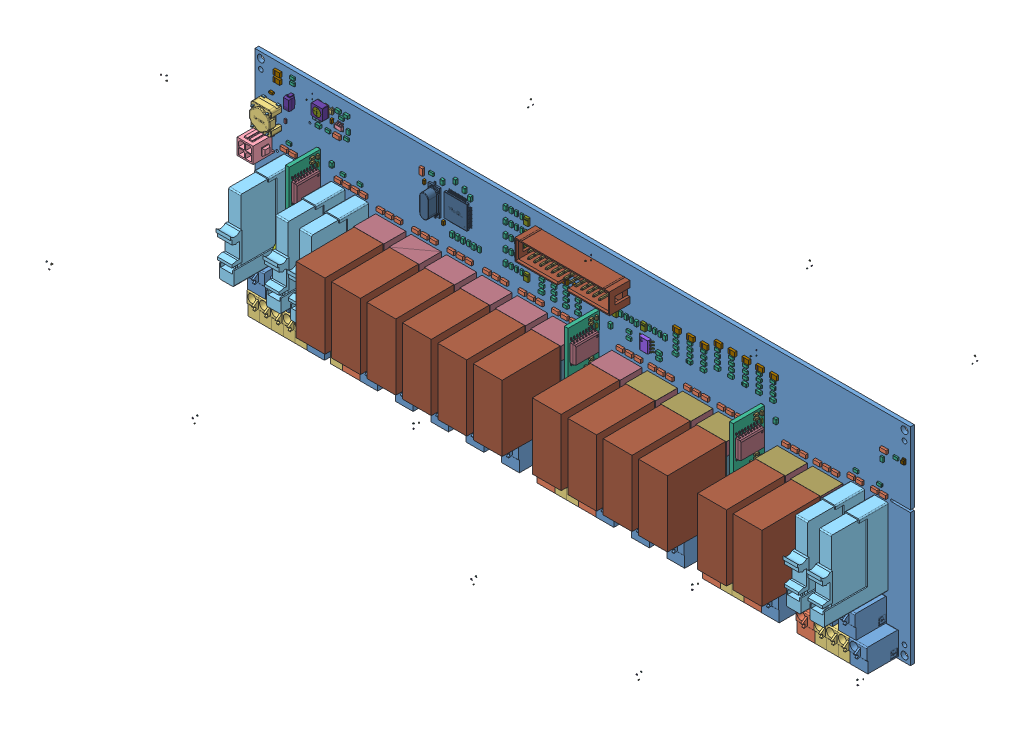
SolidWorks assembly _SC940D, configuration Default. Lengths in mm. (continued)
Components (placement in the parent): (continued)
- T25-1: T25 [Default] at origin size (306.6 73.44 23.48)
  - SW3dPS-transistor_SOT233_4-1: SW3dPS-transistor_SOT233_4 [Default] at (303.1237 70.5668 -21.9) x (1 0 0) z (0 -1 0) size (2.9 1.1 1.6)
  - SW3dPS-transistor_SOT233_5-1: SW3dPS-transistor_SOT233_5 [Default] at (0.3031 0.0706 -0.0219) x (1 0 0) z (0 -1 0) size (2.18 2.18 2.18)
  - SW3dPS-transistor_SOT233_6-1: SW3dPS-transistor_SOT233_6 [Default] at (0.0003 0.0001 0) x (1 0 0) z (0 -1 0) size (2.18 2.18 2.18)
  - SW3dPS-transistor_SOT233_7-1: SW3dPS-transistor_SOT233_7 [Default] x (1 0 0) z (0 -1 0) size (2.18 2.18 2.18)
- T24-1: T24 [Default] at origin size (298.98 73.44 23.48)
  - SW3dPS-transistor_SOT233_4-1: SW3dPS-transistor_SOT233_4 [Default] at (295.5037 70.5668 -21.9) x (1 0 0) z (0 -1 0) size (2.9 1.1 1.6)
  - SW3dPS-transistor_SOT233_5-1: SW3dPS-transistor_SOT233_5 [Default] at (0.2955 0.0706 -0.0219) x (1 0 0) z (0 -1 0) size (2.18 2.18 2.18)
  - SW3dPS-transistor_SOT233_6-1: SW3dPS-transistor_SOT233_6 [Default] at (0.0003 0.0001 0) x (1 0 0) z (0 -1 0) size (2.18 2.18 2.18)
  - SW3dPS-transistor_SOT233_7-1: SW3dPS-transistor_SOT233_7 [Default] x (1 0 0) z (0 -1 0) size (2.18 2.18 2.18)
- T27-1: T27 [Default] at origin size (320.25 73.44 23.48)
  - SW3dPS-transistor_SOT233_4-1: SW3dPS-transistor_SOT233_4 [Default] at (316.7762 70.5668 -21.9) x (1 0 0) z (0 -1 0) size (2.9 1.1 1.6)
  - SW3dPS-transistor_SOT233_5-1: SW3dPS-transistor_SOT233_5 [Default] at (0.3168 0.0706 -0.0219) x (1 0 0) z (0 -1 0) size (2.18 2.18 2.18)
  - SW3dPS-transistor_SOT233_6-1: SW3dPS-transistor_SOT233_6 [Default] at (0.0003 0.0001 0) x (1 0 0) z (0 -1 0) size (2.18 2.18 2.18)
  - SW3dPS-transistor_SOT233_7-1: SW3dPS-transistor_SOT233_7 [Default] x (1 0 0) z (0 -1 0) size (2.18 2.18 2.18)
- T26-1: T26 [Default] at origin size (312.63 73.44 23.48)
  - SW3dPS-transistor_SOT233_4-1: SW3dPS-transistor_SOT233_4 [Default] at (309.1562 70.5668 -21.9) x (1 0 0) z (0 -1 0) size (2.9 1.1 1.6)
  - SW3dPS-transistor_SOT233_5-1: SW3dPS-transistor_SOT233_5 [Default] at (0.3092 0.0706 -0.0219) x (1 0 0) z (0 -1 0) size (2.18 2.18 2.18)
  - SW3dPS-transistor_SOT233_6-1: SW3dPS-transistor_SOT233_6 [Default] at (0.0003 0.0001 0) x (1 0 0) z (0 -1 0) size (2.18 2.18 2.18)
  - SW3dPS-transistor_SOT233_7-1: SW3dPS-transistor_SOT233_7 [Default] x (1 0 0) z (0 -1 0) size (2.18 2.18 2.18)
- D42-1: D42 [Default] at origin size (185.97 29.62 23.48)
  - SW3dPS-transistor_SOT233_4-1: SW3dPS-transistor_SOT233_4 [Default] at (182.6513 26.7469 -21.9) x (-1 0 0) z (0 1 0) size (2.9 1.1 1.6)
  - SW3dPS-transistor_SOT233_5-1: SW3dPS-transistor_SOT233_5 [Default] at (0.1827 0.0267 -0.0219) x (-1 0 0) z (0 1 0) size (2.18 2.18 2.18)
  - SW3dPS-transistor_SOT233_6-1: SW3dPS-transistor_SOT233_6 [Default] at (0.0002 0 0) x (-1 0 0) z (0 1 0) size (2.18 2.18 2.18)
  - SW3dPS-transistor_SOT233_7-1: SW3dPS-transistor_SOT233_7 [Default] x (-1 0 0) z (0 1 0) size (2.18 2.18 2.18)
- D43-1: D43 [Default] at origin size (196.12 29.62 23.48)
  - SW3dPS-transistor_SOT233_4-1: SW3dPS-transistor_SOT233_4 [Default] at (192.8113 26.7469 -21.9) x (-1 0 0) z (0 1 0) size (2.9 1.1 1.6)
  - SW3dPS-transistor_SOT233_5-1: SW3dPS-transistor_SOT233_5 [Default] at (0.1928 0.0267 -0.0219) x (-1 0 0) z (0 1 0) size (2.18 2.18 2.18)
  - SW3dPS-transistor_SOT233_6-1: SW3dPS-transistor_SOT233_6 [Default] at (0.0002 0 0) x (-1 0 0) z (0 1 0) size (2.18 2.18 2.18)
  - SW3dPS-transistor_SOT233_7-1: SW3dPS-transistor_SOT233_7 [Default] x (-1 0 0) z (0 1 0) size (2.18 2.18 2.18)
- R74-1: R74 [Default] at origin size (2 1.2 0.7)
  - RESC2012X70N-1: RESC2012X70N [Default] at (253.2061 52.7049 0) x (-1 0 0) z (0 1 0) size (2 0.7 1.2)
- R75-1: R75 [Default] at origin size (2 1.2 0.7)
  - RESC2012X70N-1: RESC2012X70N [Default] at (263.3662 52.7049 0) x (-1 0 0) z (0 1 0) size (2 0.7 1.2)
- T28-1: T28 [Default] at origin size (327.08 75.5 23.48)
  - SW3dPS-transistor_SOT233_4-1: SW3dPS-transistor_SOT233_4 [Default] at (323.6024 72.6306 -21.9) x (1 0 0) z (0 -1 0) size (2.9 1.1 1.6)
  - SW3dPS-transistor_SOT233_5-1: SW3dPS-transistor_SOT233_5 [Default] at (0.3236 0.0726 -0.0219) x (1 0 0) z (0 -1 0) size (2.18 2.18 2.18)
  - SW3dPS-transistor_SOT233_6-1: SW3dPS-transistor_SOT233_6 [Default] at (0.0003 0.0001 0) x (1 0 0) z (0 -1 0) size (2.18 2.18 2.18)
  - SW3dPS-transistor_SOT233_7-1: SW3dPS-transistor_SOT233_7 [Default] x (1 0 0) z (0 -1 0) size (2.18 2.18 2.18)
- T29-1: T29 [Default] at origin size (337.24 75.5 23.48)
  - SW3dPS-transistor_SOT233_4-1: SW3dPS-transistor_SOT233_4 [Default] at (333.7624 72.6306 -21.9) x (1 0 0) z (0 -1 0) size (2.9 1.1 1.6)
  - SW3dPS-transistor_SOT233_5-1: SW3dPS-transistor_SOT233_5 [Default] at (0.3338 0.0726 -0.0219) x (1 0 0) z (0 -1 0) size (2.18 2.18 2.18)
  - SW3dPS-transistor_SOT233_6-1: SW3dPS-transistor_SOT233_6 [Default] at (0.0003 0.0001 0) x (1 0 0) z (0 -1 0) size (2.18 2.18 2.18)
  - SW3dPS-transistor_SOT233_7-1: SW3dPS-transistor_SOT233_7 [Default] x (1 0 0) z (0 -1 0) size (2.18 2.18 2.18)
- D7_1-1: D7_1 [Default] at origin size (64.67 29.62 23.48)
  - SW3dPS-transistor_SOT233_4-1: SW3dPS-transistor_SOT233_4 [Default] at (-61.1887 26.7469 -21.9) x (-1 0 0) z (0 1 0) size (2.9 1.1 1.6)
  - SW3dPS-transistor_SOT233_5-1: SW3dPS-transistor_SOT233_5 [Default] at (-0.0612 0.0267 -0.0219) x (-1 0 0) z (0 1 0) size (2.18 2.18 2.18)
  - SW3dPS-transistor_SOT233_6-1: SW3dPS-transistor_SOT233_6 [Default] at (-0.0001 0 0) x (-1 0 0) z (0 1 0) size (2.18 2.18 2.18)
  - SW3dPS-transistor_SOT233_7-1: SW3dPS-transistor_SOT233_7 [Default] x (-1 0 0) z (0 1 0) size (2.18 2.18 2.18)
- R6-1: R6 [Default] at origin size (2 1.2 0.7)
  - RESC2012X70N-1: RESC2012X70N [Default] at (9.3662 52.7049 0) x (-1 0 0) z (0 1 0) size (2 0.7 1.2)
- T1-1: T1 [Default] at origin size (83.24 75.5 23.48)
  - SW3dPS-transistor_SOT233_4-1: SW3dPS-transistor_SOT233_4 [Default] at (79.7624 72.6306 -21.9) x (1 0 0) z (0 -1 0) size (2.9 1.1 1.6)
  - SW3dPS-transistor_SOT233_5-1: SW3dPS-transistor_SOT233_5 [Default] at (0.0798 0.0726 -0.0219) x (1 0 0) z (0 -1 0) size (2.18 2.18 2.18)
  - SW3dPS-transistor_SOT233_6-1: SW3dPS-transistor_SOT233_6 [Default] at (0.0001 0.0001 0) x (1 0 0) z (0 -1 0) size (2.18 2.18 2.18)
  - SW3dPS-transistor_SOT233_7-1: SW3dPS-transistor_SOT233_7 [Default] x (1 0 0) z (0 -1 0) size (2.18 2.18 2.18)
- U7-1: U7 [Default] at origin size (27.38 148.76 148.76)
  - SC943-0C_20-12-2012-1: SC943-0C_20-12-2012 [Default] at (213.4696 28.0022 3.7281) x (0 1 0.000663) z (1 0 0) size (148.66 148.66 27.38)
    - Board_1-1: Board_1 [Default] at (0 0 -1.6167) size (43.5 16.8 1.62)
    - R15-1: R15 [Default] at origin size (1.6 0.8 0.55)
      - RESC1608X84N_1-1: RESC1608X84N_1 [Default] at (-0.0001 1.9049 0) x (-1 0 0) z (0 1 0) size (1.6 0.55 0.8)
    - R11-1: R11 [Default] at origin size (2 1.2 0.7)
      - RESC2012X70N_1-1: RESC2012X70N_1 [Default] at (-3.6513 -0.4763 0) x (-1 0 0) z (0 1 0) size (2 0.7 1.2)
    - R7-1: R7 [Default] at origin size (2 1.2 0.7)
      - RESC2012X70N_1-1: RESC2012X70N_1 [Default] at (-5.2388 1.5874 0) x (-1 0 0) z (0 1 0) size (2 0.7 1.2)
    - D3-1: D3 [Default] at origin size (2.6 5.2 2.43)
      - SW3dPS-DO-214AC_SMA-1: SW3dPS-DO-214AC_SMA [Default] at (-1.4287 0.3175 -2.9167) x (1 0 0) z (0 0 -1) size (2.6 5.2 2.43)
    - T4-1: T4 [Default] at origin size (6.54 9.94 2.42)
      - SW3dPS-DPAK-1-1: SW3dPS-DPAK-1 [Default] at (10.9238 2.2758 -2.8167) x (1 0 0) z (0 1 0) size (6.54 2.42 9.94)
    - T3-1: T3 [Default] at origin size (6.54 9.94 2.42)
      - SW3dPS-DPAK-1-1: SW3dPS-DPAK-1 [Default] at (-10.3487 2.2758 -2.8167) x (1 0 0) z (0 1 0) size (6.54 2.42 9.94)
    - D5-1: D5 [Default] at origin size (2.6 5.2 2.43)
      - SW3dPS-DO-214AC_SMA-1: SW3dPS-DO-214AC_SMA [Default] at (2.0638 0.3175 -2.9167) x (1 0 0) z (0 0 -1) size (2.6 5.2 2.43)
    - D4-1: D4 [Default] at origin size (2.6 5.2 2.43)
      - SW3dPS-DO-214AC_SMA-1: SW3dPS-DO-214AC_SMA [Default] at (5.2388 0.3175 -2.9167) x (1 0 0) z (0 0 -1) size (2.6 5.2 2.43)
    - D2-1: D2 [Default] at origin size (2.6 5.2 2.43)
      - SW3dPS-DO-214AC_SMA-1: SW3dPS-DO-214AC_SMA [Default] at (-4.6037 0.3175 -2.9167) x (1 0 0) z (0 0 -1) size (2.6 5.2 2.43)
    - R25-1: R25 [Default] at origin size (3.2 1.6 0.84)
      - RESC3216X84N-1: RESC3216X84N [Default] at (-2.0851 5.5563 -1.6167) x (-1 0 0) z (0 -1 0) size (3.2 0.84 1.6)
    - R26-1: R26 [Default] at origin size (3.2 1.6 0.84)
      - RESC3216X84N-1: RESC3216X84N [Default] at (2.6989 5.5562 -1.6167) x (1 0 0) z (0 1 0) size (3.2 0.84 1.6)
    - C6-1: C6 [Default] at origin size (0.8 1.6 0.9)
      - User_Library-CAPC1608X09_1-1: User_Library-CAPC1608X09_1 [Default] at (10.0013 0.1587 0) x (0 -1 0) z (0 0 1) size (1.6 0.8 0.9)
    - C7-1: C7 [Default] at origin size (0.8 1.6 0.9)
      - User_Library-CAPC1608X09_1-1: User_Library-CAPC1608X09_1 [Default] at (27.7813 0.1587 0) x (0 -1 0) z (0 0 1) size (1.6 0.8 0.9)
    - C8-1: C8 [Default] at origin size (0.8 1.6 0.9)
      - User_Library-CAPC1608X09_1-1: User_Library-CAPC1608X09_1 [Default] at (26.1938 0.1587 0) x (0 -1 0) z (0 0 1) size (1.6 0.8 0.9)
    - C9-1: C9 [Default] at origin size (1.6 0.8 0.9)
      - User_Library-CAPC1608X09_1-1: User_Library-CAPC1608X09_1 [Default] at (7.7788 2.3813 0) size (1.6 0.8 0.9)
    - L1-1: L1 [Default] at origin size (1.6 0.8 0.9)
      - User_Library-CAPC1608X09_1-1: User_Library-CAPC1608X09_1 [Default] at (10.7949 -2.0638 0) x (-1 0 0) z (0 0 1) size (1.6 0.8 0.9)
    - L2-1: L2 [Default] at origin size (1.6 0.8 0.9)
      - User_Library-CAPC1608X09_1-1: User_Library-CAPC1608X09_1 [Default] at (27.1463 -2.2224 0) size (1.6 0.8 0.9)
    - L3-1: L3 [Default] at origin size (1.6 0.8 0.9)
      - User_Library-CAPC1608X09_1-1: User_Library-CAPC1608X09_1 [Default] at (10.7949 2.3812 0) x (-1 0 0) z (0 0 1) size (1.6 0.8 0.9)
    - U1-1: U1 [Default] at origin size (10.3 10.3 2.65)
      - SW3dPS-SOIC16-300-1: SW3dPS-SOIC16-300 [Default] at (19.685 3.9689 0) x (0 1 0) z (0 0 1) size (10.3 10.3 2.65)
    - R2-1: R2 [Default] at origin size (2 1.2 0.7)
      - RESC2012X70N_1-1: RESC2012X70N_1 [Default] at (-8.7312 1.9051 0) x (1 0 0) z (0 -1 0) size (2 0.7 1.2)
    - C4-1: C4 [Default] at origin size (0.8 1.6 0.9)
      - User_Library-CAPC1608X09_1-1: User_Library-CAPC1608X09_1 [Default] at (-13.0176 7.6201 0) x (0 1 0) z (0 0 1) size (1.6 0.8 0.9)
    - T6-1: T6 [Default] at origin size (36.29 81.18 23.48)
      - SW3dPS-transistor_SOT233-1: SW3dPS-transistor_SOT233 [Default] at (-33.4193 77.6987 -21.9) x (0 1 0) z (1 0 0) size (2.9 1.1 1.6)
      - SW3dPS-transistor_SOT233_1-1: SW3dPS-transistor_SOT233_1 [Default] at (-0.0334 0.0777 -0.0219) x (0 1 0) z (1 0 0) size (2.18 2.18 2.18)
      - SW3dPS-transistor_SOT233_2-1: SW3dPS-transistor_SOT233_2 [Default] at (0 0.0001 0) x (0 1 0) z (1 0 0) size (2.18 2.18 2.18)
      - SW3dPS-transistor_SOT233_3-1: SW3dPS-transistor_SOT233_3 [Default] x (0 1 0) z (1 0 0) size (2.18 2.18 2.18)
    - U2-1: U2 [Default] at origin size (6.2 5 1.75)
      - User_Library-SOIC-8-150-1: User_Library-SOIC-8-150 [Default] at (6.9849 6.3501 1) x (0 -1 0) z (-1 0 0) size (5 1.75 6.2)
        - User_Library-SOIC-8-150_pin_SOIC_SO-150_1_1-1: User_Library-SOIC-8-150_pin_SOIC_SO-150_1_1 [Default] at (0.6 0 -2) x (-1 0 0) z (0 0 -1) size (0.4 1.1 1.1)
        - User_Library-SOIC-8-150_pin_SOIC_SO-150_1_1-2: User_Library-SOIC-8-150_pin_SOIC_SO-150_1_1 [Default] at (-0.67 0 -2) x (-1 0 0) z (0 0 -1) size (0.4 1.1 1.1)
        - User_Library-SOIC-8-150_pin_SOIC_SO-150_1_1-3: User_Library-SOIC-8-150_pin_SOIC_SO-150_1_1 [Default] at (-1.94 0 2) size (0.4 1.1 1.1)
        - User_Library-SOIC-8-150_pin_SOIC_SO-150_1_1-4: User_Library-SOIC-8-150_pin_SOIC_SO-150_1_1 [Default] at (-0.67 0 2) size (0.4 1.1 1.1)
        - User_Library-SOIC-8-150_pin_SOIC_SO-150_1_1-5: User_Library-SOIC-8-150_pin_SOIC_SO-150_1_1 [Default] at (-1.94 0 -2) x (-1 0 0) z (0 0 -1) size (0.4 1.1 1.1)
        - User_Library-SOIC-8-150_pin_SOIC_SO-150_1_1-6: User_Library-SOIC-8-150_pin_SOIC_SO-150_1_1 [Default] at (1.87 0 2) size (0.4 1.1 1.1)
        - User_Library-SOIC-8-150_SOIC_150_SOIC_5X4_1_1-1: User_Library-SOIC-8-150_SOIC_150_SOIC_5X4_1_1 [Default] at origin size (5 1.5 4)
        - User_Library-SOIC-8-150_pin_SOIC_SO-150_1_1-7: User_Library-SOIC-8-150_pin_SOIC_SO-150_1_1 [Default] at (0.6 0 2) size (0.4 1.1 1.1)
        - User_Library-SOIC-8-150_pin_SOIC_SO-150_1_1-8: User_Library-SOIC-8-150_pin_SOIC_SO-150_1_1 [Default] at (1.87 0 -2) x (-1 0 0) z (0 0 -1) size (0.4 1.1 1.1)
    - R16-1: R16 [Default] at origin size (1.2 2 0.7)
      - RESC2012X70N_1-1: RESC2012X70N_1 [Default] at (-3.1751 7.3026 0) x (0 1 0) z (1 0 0) size (2 0.7 1.2)
    - R12-1: R12 [Default] at origin size (1.2 2 0.7)
      - RESC2012X70N_1-1: RESC2012X70N_1 [Default] at (2.2226 -1.2701 0) x (0 -1 0) z (-1 0 0) size (2 0.7 1.2)
    - R9-1: R9 [Default] at origin size (1.6 0.8 0.55)
      - RESC1608X84N_1-1: RESC1608X84N_1 [Default] at (1.5874 5.5562 0) x (-1 0 0) z (0 1 0) size (1.6 0.55 0.8)
    - R8-1: R8 [Default] at origin size (2 1.2 0.7)
      - RESC2012X70N_1-1: RESC2012X70N_1 [Default] at (5.0801 -1.9049 0) x (1 0 0) z (0 -1 0) size (2 0.7 1.2)
    - C5-1: C5 [Default] at origin size (0.8 1.6 0.9)
      - User_Library-CAPC1608X09_1-1: User_Library-CAPC1608X09_1 [Default] at (11.5888 0.1587 0) x (0 -1 0) z (0 0 1) size (1.6 0.8 0.9)
    - C3-1: C3 [Default] at origin size (0.8 1.6 0.9)
      - User_Library-CAPC1608X09_1-1: User_Library-CAPC1608X09_1 [Default] at (8.4138 0.1587 0) x (0 -1 0) z (0 0 1) size (1.6 0.8 0.9)
    - C2-1: C2 [Default] at origin size (0.8 1.6 0.9)
      - User_Library-CAPC1608X09_1-1: User_Library-CAPC1608X09_1 [Default] at (13.1763 0.1587 0) x (0 -1 0) z (0 0 1) size (1.6 0.8 0.9)
    - R17-1: R17 [Default] at origin size (0.8 1.6 0.55)
      - RESC1608X84N_1-1: RESC1608X84N_1 [Default] at (-1.2701 7.6201 0) x (0 1 0) z (1 0 0) size (1.6 0.55 0.8)
    - R18-1: R18 [Default] at origin size (1.6 0.8 0.55)
      - RESC1608X84N_1-1: RESC1608X84N_1 [Default] at (-6.9851 8.2549 0) x (-1 0 0) z (0 1 0) size (1.6 0.55 0.8)
    - T5-1: T5 [Default] at origin size (82.76 20.1 23.48)
      - SW3dPS-transistor_SOT233-1: SW3dPS-transistor_SOT233 [Default] at (-79.2862 -17.2268 -21.9) x (-1 0 0) z (0 1 0) size (2.9 1.1 1.6)
      - SW3dPS-transistor_SOT233_1-1: SW3dPS-transistor_SOT233_1 [Default] at (-0.0793 -0.0172 -0.0219) x (-1 0 0) z (0 1 0) size (2.18 2.18 2.18)
      - SW3dPS-transistor_SOT233_2-1: SW3dPS-transistor_SOT233_2 [Default] at (-0.0001 0 0) x (-1 0 0) z (0 1 0) size (2.18 2.18 2.18)
      - SW3dPS-transistor_SOT233_3-1: SW3dPS-transistor_SOT233_3 [Default] x (-1 0 0) z (0 1 0) size (2.18 2.18 2.18)
    - T7-1: T7 [Default] at origin size (73.54 29.78 23.48)
      - SW3dPS-transistor_SOT233-1: SW3dPS-transistor_SOT233 [Default] at (70.0609 26.9106 -21.9) x (1 0 0) z (0 -1 0) size (2.9 1.1 1.6)
      - SW3dPS-transistor_SOT233_1-1: SW3dPS-transistor_SOT233_1 [Default] at (0.0701 0.0269 -0.0219) x (1 0 0) z (0 -1 0) size (2.18 2.18 2.18)
      - SW3dPS-transistor_SOT233_2-1: SW3dPS-transistor_SOT233_2 [Default] at (0.0001 0 0) x (1 0 0) z (0 -1 0) size (2.18 2.18 2.18)
      - SW3dPS-transistor_SOT233_3-1: SW3dPS-transistor_SOT233_3 [Default] x (1 0 0) z (0 -1 0) size (2.18 2.18 2.18)
    - C1-1: C1 [Default] at origin size (1.6 0.8 0.9)
      - User_Library-CAPC1608X09_1-1: User_Library-CAPC1608X09_1 [Default] at (27.1462 -1.9049 -1.6167) x (-1 0 0) z (0 0 -1) size (1.6 0.8 0.9)
    - R19-1: R19 [Default] at origin size (1.6 0.8 0.55)
      - RESC1608X84N_1-1: RESC1608X84N_1 [Default] at (-10.7949 8.2551 0) x (1 0 0) z (0 -1 0) size (1.6 0.55 0.8)
    - R1-1: R1 [Default] at origin size (1.6 0.8 0.55)
      - RESC1608X84N_1-1: RESC1608X84N_1 [Default] at (24.1301 -2.2224 0) x (1 0 0) z (0 -1 0) size (1.6 0.55 0.8)
    - D1-1: D1 [Default] at origin size (80.06 27.08 23.48)
      - SW3dPS-transistor_SOT233-1: SW3dPS-transistor_SOT233 [Default] at (76.5874 24.2118 -21.9) x (1 0 0) z (0 -1 0) size (2.9 1.1 1.6)
      - SW3dPS-transistor_SOT233_1-1: SW3dPS-transistor_SOT233_1 [Default] at (0.0766 0.0242 -0.0219) x (1 0 0) z (0 -1 0) size (2.18 2.18 2.18)
      - SW3dPS-transistor_SOT233_2-1: SW3dPS-transistor_SOT233_2 [Default] at (0.0001 0 0) x (1 0 0) z (0 -1 0) size (2.18 2.18 2.18)
      - SW3dPS-transistor_SOT233_3-1: SW3dPS-transistor_SOT233_3 [Default] x (1 0 0) z (0 -1 0) size (2.18 2.18 2.18)
    - D6-1: D6 [Default] at origin size (13.75 77.05 23.48)
      - SW3dPS-transistor_SOT233-1: SW3dPS-transistor_SOT233 [Default] at (10.8768 -73.5712 -21.9) x (0 -1 0) z (-1 0 0) size (2.9 1.1 1.6)
      - SW3dPS-transistor_SOT233_1-1: SW3dPS-transistor_SOT233_1 [Default] at (0.0109 -0.0736 -0.0219) x (0 -1 0) z (-1 0 0) size (2.18 2.18 2.18)
      - SW3dPS-transistor_SOT233_2-1: SW3dPS-transistor_SOT233_2 [Default] at (0 -0.0001 0) x (0 -1 0) z (-1 0 0) size (2.18 2.18 2.18)
      - SW3dPS-transistor_SOT233_3-1: SW3dPS-transistor_SOT233_3 [Default] x (0 -1 0) z (-1 0 0) size (2.18 2.18 2.18)
    - D7-1: D7 [Default] at origin size (17.72 77.05 23.48)
      - SW3dPS-transistor_SOT233-1: SW3dPS-transistor_SOT233 [Default] at (14.8456 -73.5712 -21.9) x (0 -1 0) z (-1 0 0) size (2.9 1.1 1.6)
      - SW3dPS-transistor_SOT233_1-1: SW3dPS-transistor_SOT233_1 [Default] at (0.0148 -0.0736 -0.0219) x (0 -1 0) z (-1 0 0) size (2.18 2.18 2.18)
      - SW3dPS-transistor_SOT233_2-1: SW3dPS-transistor_SOT233_2 [Default] at (0 -0.0001 0) x (0 -1 0) z (-1 0 0) size (2.18 2.18 2.18)
      - SW3dPS-transistor_SOT233_3-1: SW3dPS-transistor_SOT233_3 [Default] x (0 -1 0) z (-1 0 0) size (2.18 2.18 2.18)
    - R3-1: R3 [Default] at origin size (2 1.2 0.7)
      - RESC2012X70N_1-1: RESC2012X70N_1 [Default] at (-12.2237 1.9051 0) x (1 0 0) z (0 -1 0) size (2 0.7 1.2)
- U2_1-1: U2_1 [Default] at origin size (27.38 148.76 148.76)
  - SC943-0C_20-12-2012-1: SC943-0C_20-12-2012 [Default] at (22.4731 28.0022 3.7281) x (0 1 0.000663) z (1 0 0) size (148.66 148.66 27.38)
    - Board_1-1: Board_1 [Default] at (0 0 -1.6167) size (43.5 16.8 1.62)
    - R15-1: R15 [Default] at origin size (1.6 0.8 0.55)
      - RESC1608X84N_1-1: RESC1608X84N_1 [Default] at (-0.0001 1.9049 0) x (-1 0 0) z (0 1 0) size (1.6 0.55 0.8)
    - R11-1: R11 [Default] at origin size (2 1.2 0.7)
      - RESC2012X70N_1-1: RESC2012X70N_1 [Default] at (-3.6513 -0.4763 0) x (-1 0 0) z (0 1 0) size (2 0.7 1.2)
    - R7-1: R7 [Default] at origin size (2 1.2 0.7)
      - RESC2012X70N_1-1: RESC2012X70N_1 [Default] at (-5.2388 1.5874 0) x (-1 0 0) z (0 1 0) size (2 0.7 1.2)
    - D3-1: D3 [Default] at origin size (2.6 5.2 2.43)
      - SW3dPS-DO-214AC_SMA-1: SW3dPS-DO-214AC_SMA [Default] at (-1.4287 0.3175 -2.9167) x (1 0 0) z (0 0 -1) size (2.6 5.2 2.43)
    - T4-1: T4 [Default] at origin size (6.54 9.94 2.42)
      - SW3dPS-DPAK-1-1: SW3dPS-DPAK-1 [Default] at (10.9238 2.2758 -2.8167) x (1 0 0) z (0 1 0) size (6.54 2.42 9.94)
    - T3-1: T3 [Default] at origin size (6.54 9.94 2.42)
      - SW3dPS-DPAK-1-1: SW3dPS-DPAK-1 [Default] at (-10.3487 2.2758 -2.8167) x (1 0 0) z (0 1 0) size (6.54 2.42 9.94)
    - D5-1: D5 [Default] at origin size (2.6 5.2 2.43)
      - SW3dPS-DO-214AC_SMA-1: SW3dPS-DO-214AC_SMA [Default] at (2.0638 0.3175 -2.9167) x (1 0 0) z (0 0 -1) size (2.6 5.2 2.43)
    - D4-1: D4 [Default] at origin size (2.6 5.2 2.43)
      - SW3dPS-DO-214AC_SMA-1: SW3dPS-DO-214AC_SMA [Default] at (5.2388 0.3175 -2.9167) x (1 0 0) z (0 0 -1) size (2.6 5.2 2.43)
    - D2-1: D2 [Default] at origin size (2.6 5.2 2.43)
      - SW3dPS-DO-214AC_SMA-1: SW3dPS-DO-214AC_SMA [Default] at (-4.6037 0.3175 -2.9167) x (1 0 0) z (0 0 -1) size (2.6 5.2 2.43)
    - R25-1: R25 [Default] at origin size (3.2 1.6 0.84)
      - RESC3216X84N-1: RESC3216X84N [Default] at (-2.0851 5.5563 -1.6167) x (-1 0 0) z (0 -1 0) size (3.2 0.84 1.6)
    - R26-1: R26 [Default] at origin size (3.2 1.6 0.84)
      - RESC3216X84N-1: RESC3216X84N [Default] at (2.6989 5.5562 -1.6167) x (1 0 0) z (0 1 0) size (3.2 0.84 1.6)
    - C6-1: C6 [Default] at origin size (0.8 1.6 0.9)
      - User_Library-CAPC1608X09_1-1: User_Library-CAPC1608X09_1 [Default] at (10.0013 0.1587 0) x (0 -1 0) z (0 0 1) size (1.6 0.8 0.9)
    - C7-1: C7 [Default] at origin size (0.8 1.6 0.9)
      - User_Library-CAPC1608X09_1-1: User_Library-CAPC1608X09_1 [Default] at (27.7813 0.1587 0) x (0 -1 0) z (0 0 1) size (1.6 0.8 0.9)
    - C8-1: C8 [Default] at origin size (0.8 1.6 0.9)
      - User_Library-CAPC1608X09_1-1: User_Library-CAPC1608X09_1 [Default] at (26.1938 0.1587 0) x (0 -1 0) z (0 0 1) size (1.6 0.8 0.9)
    - C9-1: C9 [Default] at origin size (1.6 0.8 0.9)
      - User_Library-CAPC1608X09_1-1: User_Library-CAPC1608X09_1 [Default] at (7.7788 2.3813 0) size (1.6 0.8 0.9)
    - L1-1: L1 [Default] at origin size (1.6 0.8 0.9)
      - User_Library-CAPC1608X09_1-1: User_Library-CAPC1608X09_1 [Default] at (10.7949 -2.0638 0) x (-1 0 0) z (0 0 1) size (1.6 0.8 0.9)
    - L2-1: L2 [Default] at origin size (1.6 0.8 0.9)
      - User_Library-CAPC1608X09_1-1: User_Library-CAPC1608X09_1 [Default] at (27.1463 -2.2224 0) size (1.6 0.8 0.9)
    - L3-1: L3 [Default] at origin size (1.6 0.8 0.9)
      - User_Library-CAPC1608X09_1-1: User_Library-CAPC1608X09_1 [Default] at (10.7949 2.3812 0) x (-1 0 0) z (0 0 1) size (1.6 0.8 0.9)
    - U1-1: U1 [Default] at origin size (10.3 10.3 2.65)
      - SW3dPS-SOIC16-300-1: SW3dPS-SOIC16-300 [Default] at (19.685 3.9689 0) x (0 1 0) z (0 0 1) size (10.3 10.3 2.65)
    - R2-1: R2 [Default] at origin size (2 1.2 0.7)
      - RESC2012X70N_1-1: RESC2012X70N_1 [Default] at (-8.7312 1.9051 0) x (1 0 0) z (0 -1 0) size (2 0.7 1.2)
    - C4-1: C4 [Default] at origin size (0.8 1.6 0.9)
      - User_Library-CAPC1608X09_1-1: User_Library-CAPC1608X09_1 [Default] at (-13.0176 7.6201 0) x (0 1 0) z (0 0 1) size (1.6 0.8 0.9)
    - T6-1: T6 [Default] at origin size (36.29 81.18 23.48)
      - SW3dPS-transistor_SOT233-1: SW3dPS-transistor_SOT233 [Default] at (-33.4193 77.6987 -21.9) x (0 1 0) z (1 0 0) size (2.9 1.1 1.6)
      - SW3dPS-transistor_SOT233_1-1: SW3dPS-transistor_SOT233_1 [Default] at (-0.0334 0.0777 -0.0219) x (0 1 0) z (1 0 0) size (2.18 2.18 2.18)
      - SW3dPS-transistor_SOT233_2-1: SW3dPS-transistor_SOT233_2 [Default] at (0 0.0001 0) x (0 1 0) z (1 0 0) size (2.18 2.18 2.18)
      - SW3dPS-transistor_SOT233_3-1: SW3dPS-transistor_SOT233_3 [Default] x (0 1 0) z (1 0 0) size (2.18 2.18 2.18)
    - U2-1: U2 [Default] at origin size (6.2 5 1.75)
      - User_Library-SOIC-8-150-1: User_Library-SOIC-8-150 [Default] at (6.9849 6.3501 1) x (0 -1 0) z (-1 0 0) size (5 1.75 6.2)
        - User_Library-SOIC-8-150_pin_SOIC_SO-150_1_1-1: User_Library-SOIC-8-150_pin_SOIC_SO-150_1_1 [Default] at (0.6 0 -2) x (-1 0 0) z (0 0 -1) size (0.4 1.1 1.1)
        - User_Library-SOIC-8-150_pin_SOIC_SO-150_1_1-2: User_Library-SOIC-8-150_pin_SOIC_SO-150_1_1 [Default] at (-0.67 0 -2) x (-1 0 0) z (0 0 -1) size (0.4 1.1 1.1)
        - User_Library-SOIC-8-150_pin_SOIC_SO-150_1_1-3: User_Library-SOIC-8-150_pin_SOIC_SO-150_1_1 [Default] at (-1.94 0 2) size (0.4 1.1 1.1)
        - User_Library-SOIC-8-150_pin_SOIC_SO-150_1_1-4: User_Library-SOIC-8-150_pin_SOIC_SO-150_1_1 [Default] at (-0.67 0 2) size (0.4 1.1 1.1)
        - User_Library-SOIC-8-150_pin_SOIC_SO-150_1_1-5: User_Library-SOIC-8-150_pin_SOIC_SO-150_1_1 [Default] at (-1.94 0 -2) x (-1 0 0) z (0 0 -1) size (0.4 1.1 1.1)
        - User_Library-SOIC-8-150_pin_SOIC_SO-150_1_1-6: User_Library-SOIC-8-150_pin_SOIC_SO-150_1_1 [Default] at (1.87 0 2) size (0.4 1.1 1.1)
        - User_Library-SOIC-8-150_SOIC_150_SOIC_5X4_1_1-1: User_Library-SOIC-8-150_SOIC_150_SOIC_5X4_1_1 [Default] at origin size (5 1.5 4)
        - User_Library-SOIC-8-150_pin_SOIC_SO-150_1_1-7: User_Library-SOIC-8-150_pin_SOIC_SO-150_1_1 [Default] at (0.6 0 2) size (0.4 1.1 1.1)
        - User_Library-SOIC-8-150_pin_SOIC_SO-150_1_1-8: User_Library-SOIC-8-150_pin_SOIC_SO-150_1_1 [Default] at (1.87 0 -2) x (-1 0 0) z (0 0 -1) size (0.4 1.1 1.1)
    - R16-1: R16 [Default] at origin size (1.2 2 0.7)
      - RESC2012X70N_1-1: RESC2012X70N_1 [Default] at (-3.1751 7.3026 0) x (0 1 0) z (1 0 0) size (2 0.7 1.2)
    - R12-1: R12 [Default] at origin size (1.2 2 0.7)
      - RESC2012X70N_1-1: RESC2012X70N_1 [Default] at (2.2226 -1.2701 0) x (0 -1 0) z (-1 0 0) size (2 0.7 1.2)
    - R9-1: R9 [Default] at origin size (1.6 0.8 0.55)
      - RESC1608X84N_1-1: RESC1608X84N_1 [Default] at (1.5874 5.5562 0) x (-1 0 0) z (0 1 0) size (1.6 0.55 0.8)
    - R8-1: R8 [Default] at origin size (2 1.2 0.7)
      - RESC2012X70N_1-1: RESC2012X70N_1 [Default] at (5.0801 -1.9049 0) x (1 0 0) z (0 -1 0) size (2 0.7 1.2)
    - C5-1: C5 [Default] at origin size (0.8 1.6 0.9)
      - User_Library-CAPC1608X09_1-1: User_Library-CAPC1608X09_1 [Default] at (11.5888 0.1587 0) x (0 -1 0) z (0 0 1) size (1.6 0.8 0.9)
    - C3-1: C3 [Default] at origin size (0.8 1.6 0.9)
      - User_Library-CAPC1608X09_1-1: User_Library-CAPC1608X09_1 [Default] at (8.4138 0.1587 0) x (0 -1 0) z (0 0 1) size (1.6 0.8 0.9)
    - C2-1: C2 [Default] at origin size (0.8 1.6 0.9)
      - User_Library-CAPC1608X09_1-1: User_Library-CAPC1608X09_1 [Default] at (13.1763 0.1587 0) x (0 -1 0) z (0 0 1) size (1.6 0.8 0.9)
    - R17-1: R17 [Default] at origin size (0.8 1.6 0.55)
      - RESC1608X84N_1-1: RESC1608X84N_1 [Default] at (-1.2701 7.6201 0) x (0 1 0) z (1 0 0) size (1.6 0.55 0.8)
    - R18-1: R18 [Default] at origin size (1.6 0.8 0.55)
      - RESC1608X84N_1-1: RESC1608X84N_1 [Default] at (-6.9851 8.2549 0) x (-1 0 0) z (0 1 0) size (1.6 0.55 0.8)
    - T5-1: T5 [Default] at origin size (82.76 20.1 23.48)
      - SW3dPS-transistor_SOT233-1: SW3dPS-transistor_SOT233 [Default] at (-79.2862 -17.2268 -21.9) x (-1 0 0) z (0 1 0) size (2.9 1.1 1.6)
      - SW3dPS-transistor_SOT233_1-1: SW3dPS-transistor_SOT233_1 [Default] at (-0.0793 -0.0172 -0.0219) x (-1 0 0) z (0 1 0) size (2.18 2.18 2.18)
      - SW3dPS-transistor_SOT233_2-1: SW3dPS-transistor_SOT233_2 [Default] at (-0.0001 0 0) x (-1 0 0) z (0 1 0) size (2.18 2.18 2.18)
      - SW3dPS-transistor_SOT233_3-1: SW3dPS-transistor_SOT233_3 [Default] x (-1 0 0) z (0 1 0) size (2.18 2.18 2.18)
    - T7-1: T7 [Default] at origin size (73.54 29.78 23.48)
      - SW3dPS-transistor_SOT233-1: SW3dPS-transistor_SOT233 [Default] at (70.0609 26.9106 -21.9) x (1 0 0) z (0 -1 0) size (2.9 1.1 1.6)
      - SW3dPS-transistor_SOT233_1-1: SW3dPS-transistor_SOT233_1 [Default] at (0.0701 0.0269 -0.0219) x (1 0 0) z (0 -1 0) size (2.18 2.18 2.18)
      - SW3dPS-transistor_SOT233_2-1: SW3dPS-transistor_SOT233_2 [Default] at (0.0001 0 0) x (1 0 0) z (0 -1 0) size (2.18 2.18 2.18)
      - SW3dPS-transistor_SOT233_3-1: SW3dPS-transistor_SOT233_3 [Default] x (1 0 0) z (0 -1 0) size (2.18 2.18 2.18)
    - C1-1: C1 [Default] at origin size (1.6 0.8 0.9)
      - User_Library-CAPC1608X09_1-1: User_Library-CAPC1608X09_1 [Default] at (27.1462 -1.9049 -1.6167) x (-1 0 0) z (0 0 -1) size (1.6 0.8 0.9)
    - R19-1: R19 [Default] at origin size (1.6 0.8 0.55)
      - RESC1608X84N_1-1: RESC1608X84N_1 [Default] at (-10.7949 8.2551 0) x (1 0 0) z (0 -1 0) size (1.6 0.55 0.8)
    - R1-1: R1 [Default] at origin size (1.6 0.8 0.55)
      - RESC1608X84N_1-1: RESC1608X84N_1 [Default] at (24.1301 -2.2224 0) x (1 0 0) z (0 -1 0) size (1.6 0.55 0.8)
    - D1-1: D1 [Default] at origin size (80.06 27.08 23.48)
      - SW3dPS-transistor_SOT233-1: SW3dPS-transistor_SOT233 [Default] at (76.5874 24.2118 -21.9) x (1 0 0) z (0 -1 0) size (2.9 1.1 1.6)
      - SW3dPS-transistor_SOT233_1-1: SW3dPS-transistor_SOT233_1 [Default] at (0.0766 0.0242 -0.0219) x (1 0 0) z (0 -1 0) size (2.18 2.18 2.18)
      - SW3dPS-transistor_SOT233_2-1: SW3dPS-transistor_SOT233_2 [Default] at (0.0001 0 0) x (1 0 0) z (0 -1 0) size (2.18 2.18 2.18)
      - SW3dPS-transistor_SOT233_3-1: SW3dPS-transistor_SOT233_3 [Default] x (1 0 0) z (0 -1 0) size (2.18 2.18 2.18)
    - D6-1: D6 [Default] at origin size (13.75 77.05 23.48)
      - SW3dPS-transistor_SOT233-1: SW3dPS-transistor_SOT233 [Default] at (10.8768 -73.5712 -21.9) x (0 -1 0) z (-1 0 0) size (2.9 1.1 1.6)
      - SW3dPS-transistor_SOT233_1-1: SW3dPS-transistor_SOT233_1 [Default] at (0.0109 -0.0736 -0.0219) x (0 -1 0) z (-1 0 0) size (2.18 2.18 2.18)
      - SW3dPS-transistor_SOT233_2-1: SW3dPS-transistor_SOT233_2 [Default] at (0 -0.0001 0) x (0 -1 0) z (-1 0 0) size (2.18 2.18 2.18)
      - SW3dPS-transistor_SOT233_3-1: SW3dPS-transistor_SOT233_3 [Default] x (0 -1 0) z (-1 0 0) size (2.18 2.18 2.18)
    - D7-1: D7 [Default] at origin size (17.72 77.05 23.48)
      - SW3dPS-transistor_SOT233-1: SW3dPS-transistor_SOT233 [Default] at (14.8456 -73.5712 -21.9) x (0 -1 0) z (-1 0 0) size (2.9 1.1 1.6)
      - SW3dPS-transistor_SOT233_1-1: SW3dPS-transistor_SOT233_1 [Default] at (0.0148 -0.0736 -0.0219) x (0 -1 0) z (-1 0 0) size (2.18 2.18 2.18)
      - SW3dPS-transistor_SOT233_2-1: SW3dPS-transistor_SOT233_2 [Default] at (0 -0.0001 0) x (0 -1 0) z (-1 0 0) size (2.18 2.18 2.18)
      - SW3dPS-transistor_SOT233_3-1: SW3dPS-transistor_SOT233_3 [Default] x (0 -1 0) z (-1 0 0) size (2.18 2.18 2.18)
    - R3-1: R3 [Default] at origin size (2 1.2 0.7)
      - RESC2012X70N_1-1: RESC2012X70N_1 [Default] at (-12.2237 1.9051 0) x (1 0 0) z (0 -1 0) size (2 0.7 1.2)
- J61-1: J61 [Default] at origin size (7.62 10 19.2)
  - 1790487-1: 1790487 [Default] at (201.065 -5.67 -10.6) x (0 1 0) z (1 0 0) size (10 19.2 7.62)
    - ffkdsa1-v2-7.62-1: ffkdsa1-v2-7.62 [Default] at (-15.6914 -27.508 9.12) x (0 -1 0) z (0 0 1) size (19.2 10 7.62)
- J9-1: J9 [Default] at origin size (7.62 10 19.2)
  - 1790487-1: 1790487 [Default] at (8.025 -5.67 -10.6) x (0 1 0) z (1 0 0) size (10 19.2 7.62)
    - ffkdsa1-v2-7.62-1: ffkdsa1-v2-7.62 [Default] at (-15.6914 -27.508 9.12) x (0 -1 0) z (0 0 1) size (19.2 10 7.62)
- J22-1: J22 [Default] at origin size (7.62 10 19.2)
  - 1790487-1: 1790487 [Default] at (38.505 -5.67 -10.6) x (0 1 0) z (1 0 0) size (10 19.2 7.62)
    - ffkdsa1-v2-7.62-1: ffkdsa1-v2-7.62 [Default] at (-15.6914 -27.508 9.12) x (0 -1 0) z (0 0 1) size (19.2 10 7.62)
- J7-1: J7 [Default] at origin size (6.88 10 19.2)
  - 1790348-1: 1790348 [Default] at (14.6051 -7.6199 0) x (0 1 0) z (1 0 0) size (10 19.2 6.88)
    - ffkds-v2-5.08-1: ffkds-v2-5.08 [Default] at (-23.7414 -38.158 -2.54) x (0 -1 0) z (0 0 1) size (19.2 10 6.88)
- J10-1: J10 [Default] at origin size (6.88 10 19.2)
  - 1790348-1: 1790348 [Default] at (19.6851 -7.6199 0) x (0 1 0) z (1 0 0) size (10 19.2 6.88)
    - ffkds-v2-5.08-1: ffkds-v2-5.08 [Default] at (-23.7414 -38.158 -2.54) x (0 -1 0) z (0 0 1) size (19.2 10 6.88)
- J12-1: J12 [Default] at origin size (6.88 10 19.2)
  - 1790348-1: 1790348 [Default] at (24.7651 -7.6199 0) x (0 1 0) z (1 0 0) size (10 19.2 6.88)
    - ffkds-v2-5.08-1: ffkds-v2-5.08 [Default] at (-23.7414 -38.158 -2.54) x (0 -1 0) z (0 0 1) size (19.2 10 6.88)
- J17-1: J17 [Default] at origin size (7.62 10 19.2)
  - 1790487-1: 1790487 [Default] at (23.265 -15.67 -10.6) x (0 1 0) z (1 0 0) size (10 19.2 7.62)
    - ffkdsa1-v2-7.62-1: ffkdsa1-v2-7.62 [Default] at (-15.6914 -27.508 9.12) x (0 -1 0) z (0 0 1) size (19.2 10 7.62)
- J20-1: J20 [Default] at origin size (6.88 10 19.2)
  - 1790348-1: 1790348 [Default] at (45.0851 -7.6199 0) x (0 1 0) z (1 0 0) size (10 19.2 6.88)
    - ffkds-v2-5.08-1: ffkds-v2-5.08 [Default] at (-23.7414 -38.158 -2.54) x (0 -1 0) z (0 0 1) size (19.2 10 6.88)
- J23-1: J23 [Default] at origin size (9.42 10 19.2)
  - 1790377-1: 1790377 [Default] at (52.7051 -7.6199 0) x (0 1 0) z (1 0 0) size (10 19.2 9.42)
    - ffkdsa-v2-7.62-1: ffkdsa-v2-7.62 [Default] at (-23.7414 -38.158 -5.08) x (0 -1 0) z (0 0 1) size (19.2 10 9.42)
- J25-1: J25 [Default] at origin size (7.62 10 19.2)
  - 1790487-1: 1790487 [Default] at (46.125 -15.67 -10.6) x (0 1 0) z (1 0 0) size (10 19.2 7.62)
    - ffkdsa1-v2-7.62-1: ffkdsa1-v2-7.62 [Default] at (-15.6914 -27.508 9.12) x (0 -1 0) z (0 0 1) size (19.2 10 7.62)
- J28-1: J28 [Default] at origin size (7.62 10 19.2)
  - 1790487-1: 1790487 [Default] at (61.365 -15.67 -10.6) x (0 1 0) z (1 0 0) size (10 19.2 7.62)
    - ffkdsa1-v2-7.62-1: ffkdsa1-v2-7.62 [Default] at (-15.6914 -27.508 9.12) x (0 -1 0) z (0 0 1) size (19.2 10 7.62)
- J14-1: J14 [Default] at origin size (7.62 10 19.2)
  - 1790487-1: 1790487 [Default] at (18.185 -5.67 -10.6) x (0 1 0) z (1 0 0) size (10 19.2 7.62)
    - ffkdsa1-v2-7.62-1: ffkdsa1-v2-7.62 [Default] at (-15.6914 -27.508 9.12) x (0 -1 0) z (0 0 1) size (19.2 10 7.62)
- J15-1: J15 [Default] at origin size (6.88 10 19.2)
  - 1790348-1: 1790348 [Default] at (29.8451 -7.6199 0) x (0 1 0) z (1 0 0) size (10 19.2 6.88)
    - ffkds-v2-5.08-1: ffkds-v2-5.08 [Default] at (-23.7414 -38.158 -2.54) x (0 -1 0) z (0 0 1) size (19.2 10 6.88)
- J4-1: J4 [Default] at origin size (7.62 10 19.2)
  - 1790487-1: 1790487 [Default] at (-2.135 -5.67 -10.6) x (0 1 0) z (1 0 0) size (10 19.2 7.62)
    - ffkdsa1-v2-7.62-1: ffkdsa1-v2-7.62 [Default] at (-15.6914 -27.508 9.12) x (0 -1 0) z (0 0 1) size (19.2 10 7.62)
- J5-1: J5 [Default] at origin size (6.88 10 19.2)
  - 1790348-1: 1790348 [Default] at (9.5251 -7.6199 0) x (0 1 0) z (1 0 0) size (10 19.2 6.88)
    - ffkds-v2-5.08-1: ffkds-v2-5.08 [Default] at (-23.7414 -38.158 -2.54) x (0 -1 0) z (0 0 1) size (19.2 10 6.88)
- J50-1: J50 [Default] at origin size (7.62 10 19.2)
  - 1790487-1: 1790487 [Default] at (147.725 -15.67 -10.6) x (0 1 0) z (1 0 0) size (10 19.2 7.62)
    - ffkdsa1-v2-7.62-1: ffkdsa1-v2-7.62 [Default] at (-15.6914 -27.508 9.12) x (0 -1 0) z (0 0 1) size (19.2 10 7.62)
- C22-1: C22 [Default] at origin size (0.8 1.6 0.9)
  - User_Library-CAPC1608X09-1: User_Library-CAPC1608X09 [Default] at (75.791 56.4371 0) x (0 1 0) z (0 0 1) size (1.6 0.8 0.9)
- C21-1: C21 [Default] at origin size (0.8 1.6 0.9)
  - User_Library-CAPC1608X09-1: User_Library-CAPC1608X09 [Default] at (67.5639 67.5641 0) x (0 1 0) z (0 0 1) size (1.6 0.8 0.9)
- Q1-1: Q1 [Default] at origin size (4.9 13.4 5.08)
  - SW3dPS-hc49_cystal-1: SW3dPS-hc49_cystal [Default] at (71.9811 62.9457 0) x (1 0 0) z (0 0 1) size (4.9 13.4 5.08)
- R52-1: R52 [Default] at origin size (2 1.2 0.7)
  - RESC2012X70N-1: RESC2012X70N [Default] at (175.7681 64.5161 0) x (1 0 0) z (0 -1 0) size (2 0.7 1.2)
- R59-1: R59 [Default] at origin size (2 1.2 0.7)
  - RESC2012X70N-1: RESC2012X70N [Default] at (181.7371 59.9441 0) x (1 0 0) z (0 -1 0) size (2 0.7 1.2)
- R66-1: R66 [Default] at origin size (2 1.2 0.7)
  - RESC2012X70N-1: RESC2012X70N [Default] at (187.7059 62.2139 0) x (-1 0 0) z (0 1 0) size (2 0.7 1.2)
- R68-1: R68 [Default] at origin size (2 1.2 0.7)
  - RESC2012X70N-1: RESC2012X70N [Default] at (199.6441 63.5001 0) x (1 0 0) z (0 -1 0) size (2 0.7 1.2)
- C40-1: C40 [Default] at origin size (1.6 0.8 0.9)
  - User_Library-CAPC1608X09-1: User_Library-CAPC1608X09 [Default] at (1.9051 67.9451 0) x (1 0 0) z (0 0 1) size (1.6 0.8 0.9)
- J3-1: J3 [Default] at origin size (40.68 9.1 12.1)
  - STEP-61202621621-rev1-1: STEP-61202621621-rev1 [Default] at (135.2551 70.2531 4.4377) x (1 0 0) z (0 0 1) size (40.68 9.1 12.1)
    - 61202621621-1: 61202621621 [Default] at origin size (40.68 9.1 9.1)
    - 6120xx21621_PIN-1: 6120xx21621_PIN [Default] at (-15.24 1.27 -1.875) size (0.64 0.64 11.6)
    - 6120xx21621_PIN-2: 6120xx21621_PIN [Default] at (-15.24 -1.27 -1.875) size (0.64 0.64 11.6)
    - 6120xx21621_PIN-3: 6120xx21621_PIN [Default] at (-12.7 1.27 -1.875) size (0.64 0.64 11.6)
    - 6120xx21621_PIN-4: 6120xx21621_PIN [Default] at (-10.16 1.27 -1.875) size (0.64 0.64 11.6)
    - 6120xx21621_PIN-5: 6120xx21621_PIN [Default] at (-12.7 -1.27 -1.875) size (0.64 0.64 11.6)
    - 6120xx21621_PIN-6: 6120xx21621_PIN [Default] at (-10.16 -1.27 -1.875) size (0.64 0.64 11.6)
    - 6120xx21621_PIN-7: 6120xx21621_PIN [Default] at (-7.62 1.27 -1.875) size (0.64 0.64 11.6)
    - 6120xx21621_PIN-8: 6120xx21621_PIN [Default] at (-7.62 -1.27 -1.875) size (0.64 0.64 11.6)
    - 6120xx21621_PIN-9: 6120xx21621_PIN [Default] at (-5.08 1.27 -1.875) size (0.64 0.64 11.6)
    - 6120xx21621_PIN-10: 6120xx21621_PIN [Default] at (-5.08 -1.27 -1.875) size (0.64 0.64 11.6)
    - 6120xx21621_PIN-11: 6120xx21621_PIN [Default] at (-2.54 1.27 -1.875) size (0.64 0.64 11.6)
    - 6120xx21621_PIN-12: 6120xx21621_PIN [Default] at (0 1.27 -1.875) size (0.64 0.64 11.6)
    - 6120xx21621_PIN-13: 6120xx21621_PIN [Default] at (-2.54 -1.27 -1.875) size (0.64 0.64 11.6)
    - 6120xx21621_PIN-14: 6120xx21621_PIN [Default] at (0 -1.27 -1.875) size (0.64 0.64 11.6)
    - 6120xx21621_PIN-15: 6120xx21621_PIN [Default] at (2.54 1.27 -1.875) size (0.64 0.64 11.6)
    - 6120xx21621_PIN-16: 6120xx21621_PIN [Default] at (2.54 -1.27 -1.875) size (0.64 0.64 11.6)
    - 6120xx21621_PIN-17: 6120xx21621_PIN [Default] at (5.08 1.27 -1.875) size (0.64 0.64 11.6)
    - 6120xx21621_PIN-18: 6120xx21621_PIN [Default] at (7.62 1.27 -1.875) size (0.64 0.64 11.6)
    - 6120xx21621_PIN-19: 6120xx21621_PIN [Default] at (5.08 -1.27 -1.875) size (0.64 0.64 11.6)
    - 6120xx21621_PIN-20: 6120xx21621_PIN [Default] at (7.62 -1.27 -1.875) size (0.64 0.64 11.6)
    - 6120xx21621_PIN-21: 6120xx21621_PIN [Default] at (10.16 1.27 -1.875) size (0.64 0.64 11.6)
    - 6120xx21621_PIN-22: 6120xx21621_PIN [Default] at (12.7 1.27 -1.875) size (0.64 0.64 11.6)
    - 6120xx21621_PIN-23: 6120xx21621_PIN [Default] at (10.16 -1.27 -1.875) size (0.64 0.64 11.6)
    - 6120xx21621_PIN-24: 6120xx21621_PIN [Default] at (12.7 -1.27 -1.875) size (0.64 0.64 11.6)
    - 6120xx21621_PIN-25: 6120xx21621_PIN [Default] at (15.24 1.27 -1.875) size (0.64 0.64 11.6)
    - 6120xx21621_PIN-26: 6120xx21621_PIN [Default] at (15.24 -1.27 -1.875) size (0.64 0.64 11.6)
- R79-1: R79 [Default] at origin size (0.8 1.6 0.55)
  - RESC1608X84N-1: RESC1608X84N [Default] at (7.747 60.1979 0) x (0 -1 0) z (-1 0 0) size (1.6 0.55 0.8)
- R80-1: R80 [Default] at origin size (0.8 1.6 0.55)
  - RESC1608X84N-1: RESC1608X84N [Default] at (-4.1442 60.201 0) x (0 -1 0) z (-1 0 0) size (1.6 0.55 0.8)
- R78-1: R78 [Default] at origin size (2 1.2 0.7)
  - RESC2012X70N-1: RESC2012X70N [Default] at (26.0286 65.7224 0) x (-1 0 0) z (0 1 0) size (2 0.7 1.2)
- R4-1: R4 [Default] at origin size (1.2 2 0.7)
  - RESC2012X70N-1: RESC2012X70N [Default] at (34.7981 69.6912 0) x (0 -1 0) z (-1 0 0) size (2 0.7 1.2)
- L2_1-1: L2_1 [Default] at origin size (3.2 1.6 1)
  - SW3dPS-1206_SMD_Resistor-1: SW3dPS-1206_SMD_Resistor [Default] at (21.463 68.2625 0) x (-1 0 0) z (0 1 0) size (3.2 1 1.6)
- L1_1-1: L1_1 [Default] at origin size (4.8 4.8 2.8)
  - WE-TPC_4828-1: WE-TPC_4828 [Default] at (23.6855 72.7074 2.794) x (-1 0 0) z (0 0 1) size (4.8 4.8 2.8)
    - base-1: base [Default] at origin size (2.96 2.96 2.41)
    - base_2-1: base_2 [Default] at origin size (3.46 3.46 2.62)
    - base_3-1: base_3 [Default] at origin size (4.8 4.8 2.5)
    - base_4-1: base_4 [Default] at origin size (2.76 2.76 2.41)
    - Lötstreifen-1: Lötstreifen [Default] at (0 0 -2.8) x (-1 0 0) z (0 0 -1) size (1.6 4.8 0.3)
    - Lötstreifen_1-1: Lötstreifen_1 [Default] at (0 0 -2.8) x (-1 0 0) z (0 0 -1) size (1.6 4.8 0.3)
- D4_1-1: D4_1 [Default] at origin size (45.58 45.81 23.48)
  - SW3dPS-transistor_SOT233_4-1: SW3dPS-transistor_SOT233_4 [Default] at (-42.1069 42.9394 -21.9) x (-1 0 0) z (0 1 0) size (2.9 1.1 1.6)
  - SW3dPS-transistor_SOT233_5-1: SW3dPS-transistor_SOT233_5 [Default] at (-0.0421 0.0429 -0.0219) x (-1 0 0) z (0 1 0) size (2.18 2.18 2.18)
  - SW3dPS-transistor_SOT233_6-1: SW3dPS-transistor_SOT233_6 [Default] at (0 0 0) x (-1 0 0) z (0 1 0) size (2.18 2.18 2.18)
  - SW3dPS-transistor_SOT233_7-1: SW3dPS-transistor_SOT233_7 [Default] x (-1 0 0) z (0 1 0) size (2.18 2.18 2.18)
- D6_1-1: D6_1 [Default] at origin size (1.36 2.6 1.13)
  - SW3dPS-SOD-323-1: SW3dPS-SOD-323 [Default] at (27.8129 73.9776 0) x (0 1 0) z (0 0 1) size (2.6 1.36 1.13)
- C1_1-1: C1_1 [Default] at origin size (2 1.25 1)
  - User_Library-CAPC2013X10-1: User_Library-CAPC2013X10 [Default] at (30.5116 75.4062 0) x (-1 0 0) z (0 0 1) size (2 1.25 1)
- C4_1-1: C4_1 [Default] at origin size (2 1.25 1)
  - User_Library-CAPC2013X10-1: User_Library-CAPC2013X10 [Default] at (22.0981 65.7225 0) x (1 0 0) z (0 0 1) size (2 1.25 1)
- C2_1-1: C2_1 [Default] at origin size (2 1.25 1)
  - User_Library-CAPC2013X10-1: User_Library-CAPC2013X10 [Default] at (34.1629 75.438 0) x (-1 0 0) z (0 0 1) size (2 1.25 1)
- C3_1-1: C3_1 [Default] at origin size (0.8 1.6 0.9)
  - User_Library-CAPC1608X09-1: User_Library-CAPC1608X09 [Default] at (27.8131 70.3617 0) x (0 -1 0) z (0 0 1) size (1.6 0.8 0.9)
- U1_1-1: U1_1 [Default] at origin size (3 3 1.35)
  - User_Library-SOT23-6-1: User_Library-SOT23-6 [Default] at (31.1467 69.8501 0) x (0 1 0) z (0 0 1) size (3 3 1.35)
- R3_1-1: R3_1 [Default] at origin size (2 1.2 0.7)
  - RESC2012X70N-1: RESC2012X70N [Default] at (34.0042 66.6749 0) x (-1 0 0) z (0 1 0) size (2 0.7 1.2)
- R5-1: R5 [Default] at origin size (2 1.2 0.7)
  - RESC2012X70N-1: RESC2012X70N [Default] at (31.9404 73.3424 0) x (-1 0 0) z (0 1 0) size (2 0.7 1.2)
